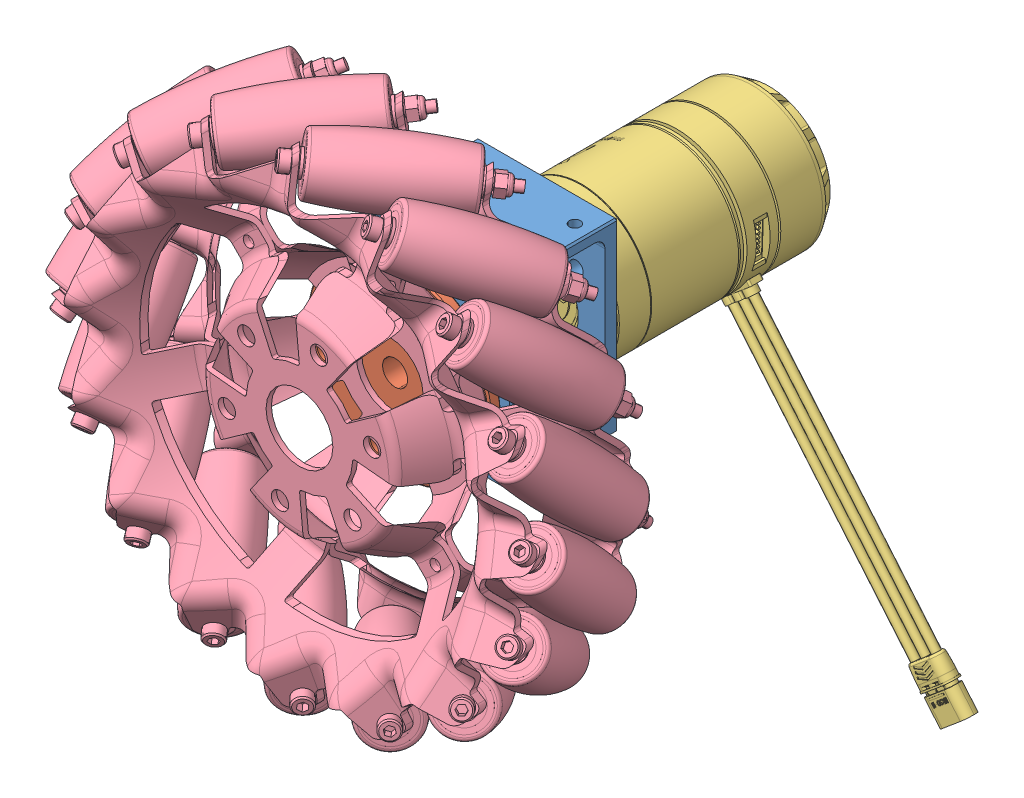
SolidWorks assembly 麦轮总装左轮, configuration 默认. Lengths in mm.
Overall size (227.85 229.28 154.75).
5 component instances, 4 part files, 3 mates.
Components (placement in the parent):
- 3508电机-1: 3508电机 [Default] at (43.0796 -3.0277 90.2458) size (124.33 157.68 116.9)
  - 电机座Z80123-1: 电机座Z80123 [默认] at (-77.6885 26.4734 96.0875) size (42 55.4 32)
  - 电机连轴Z80123-1: 电机连轴Z80123 [默认] at (-77.6885 26.4734 125.8875) x (0.707107 -0.707107 0) z (0.707107 0.707107 0) size (55 37.5 55)
  - M3508直流无刷减速电机-2: M3508直流无刷减速电机 [默认] at (-69.0293 10.2886 -6.3535) x (0.923508 0.383579 0) z (0 0 1) size (63.71 141 98.4)
- 麦轮镂空（左）-1: 麦轮镂空（左） [默认] at (-104.2541 -78.9214 138.5246) x (-0.707107 0.707107 0) z (0.707107 0.707107 0) size (178.66 47.46 178.66)
Mates (geometry in assembly coordinates):
- 重合1: coincident anti-aligned: plane of 3508电机-1/电机连轴Z80123-1 through (-34.6089 23.4456 216.1333) normal (0 0 1); plane of 麦轮镂空（左）-1 through (-30.1604 -21.7201 216.1333) normal (0 0 -1)
- 同心1: concentric anti-aligned: cylinder of 3508电机-1/电机连轴Z80123-1 through (-34.6089 23.4456 216.1333) axis (0 0 -1) radius 3.75; cylinder of 麦轮镂空（左）-1 through (-34.6089 23.4456 215.9721) axis (0 0 1) radius 10
- 同心2: concentric aligned: cylinder of 3508电机-1/电机连轴Z80123-1 through (-56.3422 17.6222 205.1333) axis (0 0 1) radius 2.6; cylinder of 麦轮镂空（左）-1 through (-56.3422 17.6222 242.9723) axis (0 0 1) radius 2.6
